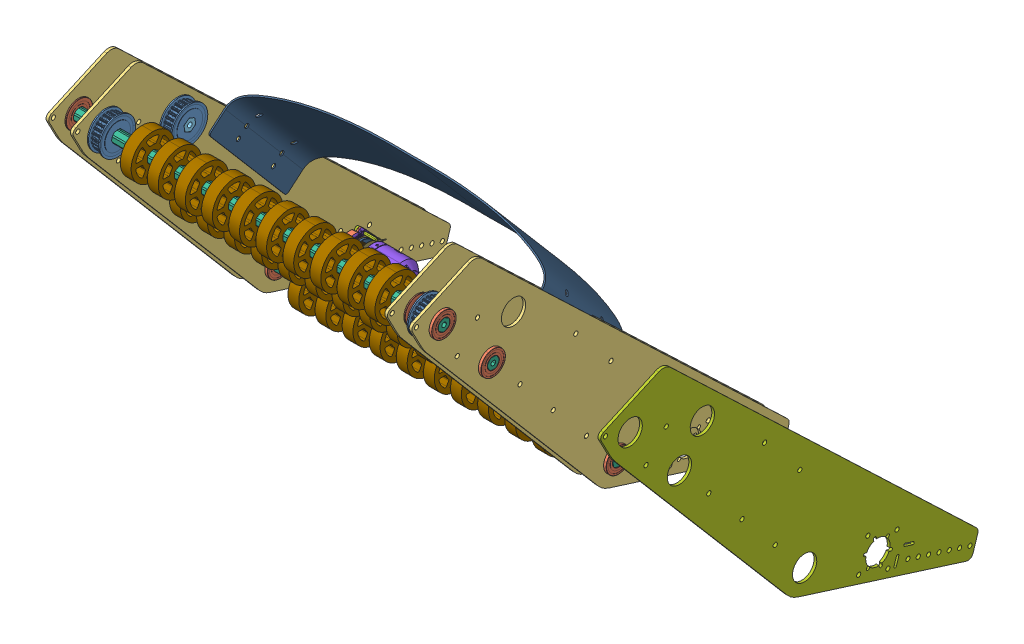
SolidWorks assembly noahbackupintake, configuration Default. Lengths in mm.
Overall size (656.48 502.65 458.04).
111 component instances, 28 part files, 0 mates.
Components (placement in the parent):
- EBUD-000_INTAKE_STEP_ASM^04_INTAKE_ASM_00_2023_everybot_asm_final_rev2(2)_00_2023_everybot_asm_final_rev2-1: EBUD-000_INTAKE_STEP_ASM^04_INTAKE_ASM_00_2023_everybot_asm_final_rev2(2)_00_2023_everybot_asm_final_rev2 [Default] at origin size (656.48 502.65 458.04) (virtual)
  - 24T_X_9MM_WIDE_DOUBLE_FLANGE_AL^EBUD-000_INTAKE_STEP_ASM_04_INTAKE_ASM_00_2023_everybot_asm_final_rev2(2)_00_2023_everybot_asm_final_rev2-1: 24T_X_9MM_WIDE_DOUBLE_FLANGE_AL^EBUD-000_INTAKE_STEP_ASM_04_INTAKE_ASM_00_2023_everybot_asm_final_rev2(2)_00_2023_everybot_asm_final_rev2 [Default] at (-209.55 741.6884 782.7658) x (0 0.711961 0.702219) z (1 0 0) size (42 42 14.5) (virtual)
  - 24T_X_9MM_WIDE_DOUBLE_FLANGE_AL^EBUD-000_INTAKE_STEP_ASM_04_INTAKE_ASM_00_2023_everybot_asm_final_rev2(2)_00_2023_everybot_asm_final_rev2-2: 24T_X_9MM_WIDE_DOUBLE_FLANGE_AL^EBUD-000_INTAKE_STEP_ASM_04_INTAKE_ASM_00_2023_everybot_asm_final_rev2(2)_00_2023_everybot_asm_final_rev2 [Default] at (-209.55 714.5782 696.9507) x (0 -0.172794 -0.984958) z (1 0 0) size (42 42 14.5) (virtual)
  - 13_75MM__1_2_THUNDERHEX_ID__X_1^EBUD-000_INTAKE_STEP_ASM_04_INTAKE_ASM_00_2023_everybot_asm_final_rev2(2)_00_2023_everybot_asm_final_rev2-1: 13_75MM__1_2_THUNDERHEX_ID__X_1^EBUD-000_INTAKE_STEP_ASM_04_INTAKE_ASM_00_2023_everybot_asm_final_rev2(2)_00_2023_everybot_asm_final_rev2 [Default] at (-224.6312 714.5782 696.9507) x (0 -0.939164 0.343468) z (1 0 0) size (31.12 31.12 7.94) (virtual)
  - 13_75MM__1_2_THUNDERHEX_ID__X_1^EBUD-000_INTAKE_STEP_ASM_04_INTAKE_ASM_00_2023_everybot_asm_final_rev2(2)_00_2023_everybot_asm_final_rev2-2: 13_75MM__1_2_THUNDERHEX_ID__X_1^EBUD-000_INTAKE_STEP_ASM_04_INTAKE_ASM_00_2023_everybot_asm_final_rev2(2)_00_2023_everybot_asm_final_rev2 [Default] at (-224.6312 741.6884 782.7658) x (0 -0.292473 -0.956274) z (1 0 0) size (31.12 31.12 7.94) (virtual)
  - 04_INTAKE_PLATE^EBUD-000_INTAKE_STEP_ASM_04_INTAKE_ASM_00_2023_everybot_asm_final_rev2(2)_00_2023_everybot_asm_final_rev2-1: 04_INTAKE_PLATE^EBUD-000_INTAKE_STEP_ASM_04_INTAKE_ASM_00_2023_everybot_asm_final_rev2(2)_00_2023_everybot_asm_final_rev2 [Default] at (-223.8375 981.3273 987.2051) x (1 0 0) z (0 -0.649023 0.760769) size (3.17 540.33 141.11) (virtual)
  - 04_INTAKE_PLATE^EBUD-000_INTAKE_STEP_ASM_04_INTAKE_ASM_00_2023_everybot_asm_final_rev2(2)_00_2023_everybot_asm_final_rev2-2: 04_INTAKE_PLATE^EBUD-000_INTAKE_STEP_ASM_04_INTAKE_ASM_00_2023_everybot_asm_final_rev2(2)_00_2023_everybot_asm_final_rev2 [Default] at (-195.2625 981.3273 987.2051) x (1 0 0) z (0 -0.649023 0.760769) size (3.17 540.33 141.11) (virtual)
  - 04_INTAKE_PLATE^EBUD-000_INTAKE_STEP_ASM_04_INTAKE_ASM_00_2023_everybot_asm_final_rev2(2)_00_2023_everybot_asm_final_rev2-3: 04_INTAKE_PLATE^EBUD-000_INTAKE_STEP_ASM_04_INTAKE_ASM_00_2023_everybot_asm_final_rev2(2)_00_2023_everybot_asm_final_rev2 [Default] at (173.1645 981.3273 987.2051) x (1 0 0) z (0 -0.649023 0.760769) size (3.17 540.33 141.11) (virtual)
  - 04_INTAKE_PLATE^EBUD-000_INTAKE_STEP_ASM_04_INTAKE_ASM_00_2023_everybot_asm_final_rev2(2)_00_2023_everybot_asm_final_rev2-4: 04_INTAKE_PLATE^EBUD-000_INTAKE_STEP_ASM_04_INTAKE_ASM_00_2023_everybot_asm_final_rev2(2)_00_2023_everybot_asm_final_rev2 [Default] at (201.7395 981.3273 987.2051) x (1 0 0) z (0 -0.649023 0.760769) size (3.17 540.33 141.11) (virtual)
  - 13_75MM__1_2_THUNDERHEX_ID__X_1^EBUD-000_INTAKE_STEP_ASM_04_INTAKE_ASM_00_2023_everybot_asm_final_rev2(2)_00_2023_everybot_asm_final_rev2-3: 13_75MM__1_2_THUNDERHEX_ID__X_1^EBUD-000_INTAKE_STEP_ASM_04_INTAKE_ASM_00_2023_everybot_asm_final_rev2(2)_00_2023_everybot_asm_final_rev2 [Default] at (-194.4688 981.3273 987.2051) x (0 0.254987 0.966944) z (-1 0 0) size (31.12 31.12 7.94) (virtual)
  - 13_75MM__1_2_THUNDERHEX_ID__X_1^EBUD-000_INTAKE_STEP_ASM_04_INTAKE_ASM_00_2023_everybot_asm_final_rev2(2)_00_2023_everybot_asm_final_rev2-4: 13_75MM__1_2_THUNDERHEX_ID__X_1^EBUD-000_INTAKE_STEP_ASM_04_INTAKE_ASM_00_2023_everybot_asm_final_rev2(2)_00_2023_everybot_asm_final_rev2 [Default] at (-224.6312 950.6568 902.5971) x (0 0.861369 0.50798) z (1 0 0) size (31.12 31.12 7.94) (virtual)
  - 13_75MM__1_2_THUNDERHEX_ID__X_1^EBUD-000_INTAKE_STEP_ASM_04_INTAKE_ASM_00_2023_everybot_asm_final_rev2(2)_00_2023_everybot_asm_final_rev2-5: 13_75MM__1_2_THUNDERHEX_ID__X_1^EBUD-000_INTAKE_STEP_ASM_04_INTAKE_ASM_00_2023_everybot_asm_final_rev2(2)_00_2023_everybot_asm_final_rev2 [Default] at (-224.6312 981.3273 987.2051) x (0 0.96991 0.243463) z (1 0 0) size (31.12 31.12 7.94) (virtual)
  - 24T_X_9MM_WIDE_DOUBLE_FLANGE_AL^EBUD-000_INTAKE_STEP_ASM_04_INTAKE_ASM_00_2023_everybot_asm_final_rev2(2)_00_2023_everybot_asm_final_rev2-3: 24T_X_9MM_WIDE_DOUBLE_FLANGE_AL^EBUD-000_INTAKE_STEP_ASM_04_INTAKE_ASM_00_2023_everybot_asm_final_rev2(2)_00_2023_everybot_asm_final_rev2 [Default] at (-183.25 981.3273 987.2051) x (0 -0.068988 0.997618) z (1 0 0) size (42 42 14.5) (virtual)
  - 13_75MM__1_2_THUNDERHEX_ID__X_1^EBUD-000_INTAKE_STEP_ASM_04_INTAKE_ASM_00_2023_everybot_asm_final_rev2(2)_00_2023_everybot_asm_final_rev2-6: 13_75MM__1_2_THUNDERHEX_ID__X_1^EBUD-000_INTAKE_STEP_ASM_04_INTAKE_ASM_00_2023_everybot_asm_final_rev2(2)_00_2023_everybot_asm_final_rev2 [Default] at (-194.4688 913.695 929.507) x (0 0.294166 0.955754) z (-1 0 0) size (31.12 31.12 7.94) (virtual)
  - 13_75MM__1_2_THUNDERHEX_ID__X_1^EBUD-000_INTAKE_STEP_ASM_04_INTAKE_ASM_00_2023_everybot_asm_final_rev2(2)_00_2023_everybot_asm_final_rev2-7: 13_75MM__1_2_THUNDERHEX_ID__X_1^EBUD-000_INTAKE_STEP_ASM_04_INTAKE_ASM_00_2023_everybot_asm_final_rev2(2)_00_2023_everybot_asm_final_rev2 [Default] at (-224.6312 913.695 929.507) x (0 0.91904 0.394165) z (1 0 0) size (31.12 31.12 7.94) (virtual)
  - REV-21-1929^EBUD-000_INTAKE_STEP_ASM_04_INTAKE_ASM_00_2023_everybot_asm_final_rev2(2)_00_2023_everybot_asm_final_rev2-1: REV-21-1929^EBUD-000_INTAKE_STEP_ASM_04_INTAKE_ASM_00_2023_everybot_asm_final_rev2(2)_00_2023_everybot_asm_final_rev2 [Default] at (-209.55 913.695 929.507) x (0 0 1) z (-1 0 0) size (48.2 48.2 12.7) (virtual)
  - 13_75MM__1_2_THUNDERHEX_ID__X_1^EBUD-000_INTAKE_STEP_ASM_04_INTAKE_ASM_00_2023_everybot_asm_final_rev2(2)_00_2023_everybot_asm_final_rev2-8: 13_75MM__1_2_THUNDERHEX_ID__X_1^EBUD-000_INTAKE_STEP_ASM_04_INTAKE_ASM_00_2023_everybot_asm_final_rev2(2)_00_2023_everybot_asm_final_rev2 [Default] at (-194.4688 741.6884 782.7658) x (0 -0.454664 -0.890663) z (-1 0 0) size (31.12 31.12 7.94) (virtual)
  - REV-21-1929^EBUD-000_INTAKE_STEP_ASM_04_INTAKE_ASM_00_2023_everybot_asm_final_rev2(2)_00_2023_everybot_asm_final_rev2-2: REV-21-1929^EBUD-000_INTAKE_STEP_ASM_04_INTAKE_ASM_00_2023_everybot_asm_final_rev2(2)_00_2023_everybot_asm_final_rev2 [Default] at (-209.55 950.6568 902.5971) x (0 0.397418 0.917638) z (-1 0 0) size (48.2 48.2 12.7) (virtual)
  - 13_75MM__1_2_THUNDERHEX_ID__X_1^EBUD-000_INTAKE_STEP_ASM_04_INTAKE_ASM_00_2023_everybot_asm_final_rev2(2)_00_2023_everybot_asm_final_rev2-9: 13_75MM__1_2_THUNDERHEX_ID__X_1^EBUD-000_INTAKE_STEP_ASM_04_INTAKE_ASM_00_2023_everybot_asm_final_rev2(2)_00_2023_everybot_asm_final_rev2 [Default] at (-194.4688 950.6568 902.5971) x (0 0.163432 0.986555) z (-1 0 0) size (31.12 31.12 7.94) (virtual)
  - 24T_X_9MM_WIDE_DOUBLE_FLANGE_AL^EBUD-000_INTAKE_STEP_ASM_04_INTAKE_ASM_00_2023_everybot_asm_final_rev2(2)_00_2023_everybot_asm_final_rev2-4: 24T_X_9MM_WIDE_DOUBLE_FLANGE_AL^EBUD-000_INTAKE_STEP_ASM_04_INTAKE_ASM_00_2023_everybot_asm_final_rev2(2)_00_2023_everybot_asm_final_rev2 [Default] at (-183.25 950.6568 902.5971) x (0 0.99517 0.098168) z (1 0 0) size (42 42 14.5) (virtual)
  - 13_75MM__1_2_THUNDERHEX_ID__X_1^EBUD-000_INTAKE_STEP_ASM_04_INTAKE_ASM_00_2023_everybot_asm_final_rev2(2)_00_2023_everybot_asm_final_rev2-10: 13_75MM__1_2_THUNDERHEX_ID__X_1^EBUD-000_INTAKE_STEP_ASM_04_INTAKE_ASM_00_2023_everybot_asm_final_rev2(2)_00_2023_everybot_asm_final_rev2 [Default] at (172.3707 913.695 929.507) x (0 -0.294166 -0.955754) z (1 0 0) size (31.12 31.12 7.94) (virtual)
  - 13_75MM__1_2_THUNDERHEX_ID__X_1^EBUD-000_INTAKE_STEP_ASM_04_INTAKE_ASM_00_2023_everybot_asm_final_rev2(2)_00_2023_everybot_asm_final_rev2-11: 13_75MM__1_2_THUNDERHEX_ID__X_1^EBUD-000_INTAKE_STEP_ASM_04_INTAKE_ASM_00_2023_everybot_asm_final_rev2(2)_00_2023_everybot_asm_final_rev2 [Default] at (172.3707 741.6884 782.7658) x (0 0.454664 0.890663) z (1 0 0) size (31.12 31.12 7.94) (virtual)
  - 13_75MM__1_2_THUNDERHEX_ID__X_1^EBUD-000_INTAKE_STEP_ASM_04_INTAKE_ASM_00_2023_everybot_asm_final_rev2(2)_00_2023_everybot_asm_final_rev2-12: 13_75MM__1_2_THUNDERHEX_ID__X_1^EBUD-000_INTAKE_STEP_ASM_04_INTAKE_ASM_00_2023_everybot_asm_final_rev2(2)_00_2023_everybot_asm_final_rev2 [Default] at (202.5333 981.3273 987.2051) x (0 -0.96991 -0.243463) z (-1 0 0) size (31.12 31.12 7.94) (virtual)
  - 13_75MM__1_2_THUNDERHEX_ID__X_1^EBUD-000_INTAKE_STEP_ASM_04_INTAKE_ASM_00_2023_everybot_asm_final_rev2(2)_00_2023_everybot_asm_final_rev2-13: 13_75MM__1_2_THUNDERHEX_ID__X_1^EBUD-000_INTAKE_STEP_ASM_04_INTAKE_ASM_00_2023_everybot_asm_final_rev2(2)_00_2023_everybot_asm_final_rev2 [Default] at (202.5333 913.695 929.507) x (0 -0.91904 -0.394165) z (-1 0 0) size (31.12 31.12 7.94) (virtual)
  - 13_75MM__1_2_THUNDERHEX_ID__X_1^EBUD-000_INTAKE_STEP_ASM_04_INTAKE_ASM_00_2023_everybot_asm_final_rev2(2)_00_2023_everybot_asm_final_rev2-14: 13_75MM__1_2_THUNDERHEX_ID__X_1^EBUD-000_INTAKE_STEP_ASM_04_INTAKE_ASM_00_2023_everybot_asm_final_rev2(2)_00_2023_everybot_asm_final_rev2 [Default] at (202.5333 741.6884 782.7658) x (0 0.292473 0.956274) z (-1 0 0) size (31.12 31.12 7.94) (virtual)
  - 13_75MM__1_2_THUNDERHEX_ID__X_1^EBUD-000_INTAKE_STEP_ASM_04_INTAKE_ASM_00_2023_everybot_asm_final_rev2(2)_00_2023_everybot_asm_final_rev2-15: 13_75MM__1_2_THUNDERHEX_ID__X_1^EBUD-000_INTAKE_STEP_ASM_04_INTAKE_ASM_00_2023_everybot_asm_final_rev2(2)_00_2023_everybot_asm_final_rev2 [Default] at (172.3707 981.3273 987.2051) x (0 -0.254987 -0.966944) z (1 0 0) size (31.12 31.12 7.94) (virtual)
  - 04_CLUSTER_SHAFT^EBUD-000_INTAKE_STEP_ASM_04_INTAKE_ASM_00_2023_everybot_asm_final_rev2(2)_00_2023_everybot_asm_final_rev2-1: 04_CLUSTER_SHAFT^EBUD-000_INTAKE_STEP_ASM_04_INTAKE_ASM_00_2023_everybot_asm_final_rev2(2)_00_2023_everybot_asm_final_rev2 [Default] at (-190.605 950.6568 902.5971) x (1 0 0) z (0 0.754856 0.65589) size (55.88 13.76 12.7) (virtual)
  - 24T_X_9MM_WIDE_DOUBLE_FLANGE_AL^EBUD-000_INTAKE_STEP_ASM_04_INTAKE_ASM_00_2023_everybot_asm_final_rev2(2)_00_2023_everybot_asm_final_rev2-5: 24T_X_9MM_WIDE_DOUBLE_FLANGE_AL^EBUD-000_INTAKE_STEP_ASM_04_INTAKE_ASM_00_2023_everybot_asm_final_rev2(2)_00_2023_everybot_asm_final_rev2 [Default] at (191.3145 741.6884 782.7658) x (0 -0.01901 0.999819) z (1 0 0) size (42 42 14.5) (virtual)
  - 24T_X_9MM_WIDE_DOUBLE_FLANGE_AL^EBUD-000_INTAKE_STEP_ASM_04_INTAKE_ASM_00_2023_everybot_asm_final_rev2(2)_00_2023_everybot_asm_final_rev2-6: 24T_X_9MM_WIDE_DOUBLE_FLANGE_AL^EBUD-000_INTAKE_STEP_ASM_04_INTAKE_ASM_00_2023_everybot_asm_final_rev2(2)_00_2023_everybot_asm_final_rev2 [Default] at (191.3145 981.3273 987.2051) x (0 -0.068988 0.997618) z (1 0 0) size (42 42 14.5) (virtual)
  - 04_INTAKE_ROLLER_SHAFT^EBUD-000_INTAKE_STEP_ASM_04_INTAKE_ASM_00_2023_everybot_asm_final_rev2(2)_00_2023_everybot_asm_final_rev2-1: 04_INTAKE_ROLLER_SHAFT^EBUD-000_INTAKE_STEP_ASM_04_INTAKE_ASM_00_2023_everybot_asm_final_rev2(2)_00_2023_everybot_asm_final_rev2 [Default] at (-37.973 741.6873 782.7662) x (1 0 0) z (0 -0.958269 0.285869) size (435.1 13.76 12.7) (virtual)
  - 04_INTAKE_ROLLER_SHAFT^EBUD-000_INTAKE_STEP_ASM_04_INTAKE_ASM_00_2023_everybot_asm_final_rev2(2)_00_2023_everybot_asm_final_rev2-2: 04_INTAKE_ROLLER_SHAFT^EBUD-000_INTAKE_STEP_ASM_04_INTAKE_ASM_00_2023_everybot_asm_final_rev2(2)_00_2023_everybot_asm_final_rev2 [Default] at (-37.973 913.695 929.507) x (1 0 0) z (0 -0.53426 -0.84532) size (435.1 13.76 12.7) (virtual)
  - 04_INTAKE_ROLLER_SHAFT^EBUD-000_INTAKE_STEP_ASM_04_INTAKE_ASM_00_2023_everybot_asm_final_rev2(2)_00_2023_everybot_asm_final_rev2-3: 04_INTAKE_ROLLER_SHAFT^EBUD-000_INTAKE_STEP_ASM_04_INTAKE_ASM_00_2023_everybot_asm_final_rev2(2)_00_2023_everybot_asm_final_rev2 [Default] at (-37.973 981.3273 987.2051) size (435.1 13.76 12.7) (virtual)
  - 04_INTAKE_PLATE_REV2_REF_ONLY^EBUD-000_INTAKE_STEP_ASM_04_INTAKE_ASM_00_2023_everybot_asm_final_rev2(2)_00_2023_everybot_asm_final_rev2-1: 04_INTAKE_PLATE_REV2_REF_ONLY^EBUD-000_INTAKE_STEP_ASM_04_INTAKE_ASM_00_2023_everybot_asm_final_rev2(2)_00_2023_everybot_asm_final_rev2 [Default] at (423.0079 981.3273 987.2051) x (1 0 0) z (0 -0.649023 0.760769) size (3.17 540.33 141.11) (virtual)
- REV_ULTRAPLANETARY_1-STAGE_ASM^04_INTAKE_ASM_00_2023_everybot_asm_final_rev2(2)_00_2023_everybot_asm_final_rev2-1: REV_ULTRAPLANETARY_1-STAGE_ASM^04_INTAKE_ASM_00_2023_everybot_asm_final_rev2(2)_00_2023_everybot_asm_final_rev2 [Default] at (-167.425 714.5782 696.9507) x (0 -0.976417 -0.215894) z (1 0 0) size (56.74 54.7 105.61) (virtual)
  - REV_ULTRAPLANETARY__CONFIGURABL_ASM^REV_ULTRAPLANETARY_1-STAGE_ASM_04_INTAKE_ASM_00_2023_everybot_asm_final_rev2(2)_00_2023_everybot_asm_final_rev2-1: REV_ULTRAPLANETARY__CONFIGURABL_ASM^REV_ULTRAPLANETARY_1-STAGE_ASM_04_INTAKE_ASM_00_2023_everybot_asm_final_rev2(2)_00_2023_everybot_asm_final_rev2 [Default] at origin size (56.74 54.7 105.61) (virtual)
    - REV_PLANETARY_STAGE__1__ASM^REV_ULTRAPLANETARY__CONFIGURABL_ASM_REV_ULTRAPLANETARY_1-STAGE_ASM_04_INTAKE_ASM_00_2023_everybot_asm_final_rev2(2)_00_2023_everybot_asm_final_rev2-1: REV_PLANETARY_STAGE__1__ASM^REV_ULTRAPLANETARY__CONFIGURABL_ASM_REV_ULTRAPLANETARY_1-STAGE_ASM_04_INTAKE_ASM_00_2023_everybot_asm_final_rev2(2)_00_2023_everybot_asm_final_rev2 [Default] at origin size (47.64 47.49 16.75) (virtual)
      - REV_ULTRAPLANETARY_3_1_CARTRIDG_ASM^REV_PLANETARY_STAGE__1__ASM_REV_ULTRAPLANETARY__CONFIGURABL_ASM_REV_ULTRAPLANETARY_1-STAGE_ASM_04_INTAKE_ASM_00_2023_everybot_asm_final_rev2(2)_00_2023~-1: REV_ULTRAPLANETARY_3_1_CARTRIDG_ASM^REV_PLANETARY_STAGE__1__ASM_REV_ULTRAPLANETARY__CONFIGURABL_ASM_REV_ULTRAPLANETARY_1-STAGE_ASM_04_INTAKE_ASM_00_2023_everybot_asm_final_rev2(2)_00_2023_~ [Default] at origin size (47.64 47.49 16.75) (virtual)
        - REV-40-1613^REV_ULTRAPLANETARY_3_1_CARTRIDG_ASM_REV_PLANETARY_STAGE__1__ASM_REV_ULTRAPLANETARY__CONFIGURABL_ASM_REV_ULTRAPLANETARY_1-STAGE_ASM_04_INTAKE_ASM_00_2023_everybot_asm_final_rev2~-1: REV-40-1613^REV_ULTRAPLANETARY_3_1_CARTRIDG_ASM_REV_PLANETARY_STAGE__1__ASM_REV_ULTRAPLANETARY__CONFIGURABL_ASM_REV_ULTRAPLANETARY_1-STAGE_ASM_04_INTAKE_ASM_00_2023_everybot_asm_final_rev2~ [Default] at (-0.89 11.5157 -14.625) x (0 0 1) z (-0.923728 -0.383049 0) size (9 3 3) (virtual)
        - REV-41-1601-2^REV_ULTRAPLANETARY_3_1_CARTRIDG_ASM_REV_PLANETARY_STAGE__1__ASM_REV_ULTRAPLANETARY__CONFIGURABL_ASM_REV_ULTRAPLANETARY_1-STAGE_ASM_04_INTAKE_ASM_00_2023_everybot_asm_final_re~-1: REV-41-1601-2^REV_ULTRAPLANETARY_3_1_CARTRIDG_ASM_REV_PLANETARY_STAGE__1__ASM_REV_ULTRAPLANETARY__CONFIGURABL_ASM_REV_ULTRAPLANETARY_1-STAGE_ASM_04_INTAKE_ASM_00_2023_everybot_asm_final_re~ [Default] at (-0.89 11.5157 -8.625) x (0.281273 0.959628 0) z (0.959628 -0.281273 0) size (8.22 6.01 8.17) (virtual)
        - REV-41-1601-2^REV_ULTRAPLANETARY_3_1_CARTRIDG_ASM_REV_PLANETARY_STAGE__1__ASM_REV_ULTRAPLANETARY__CONFIGURABL_ASM_REV_ULTRAPLANETARY_1-STAGE_ASM_04_INTAKE_ASM_00_2023_everybot_asm_final_re~-2: REV-41-1601-2^REV_ULTRAPLANETARY_3_1_CARTRIDG_ASM_REV_PLANETARY_STAGE__1__ASM_REV_ULTRAPLANETARY__CONFIGURABL_ASM_REV_ULTRAPLANETARY_1-STAGE_ASM_04_INTAKE_ASM_00_2023_everybot_asm_final_re~ [Default] at (-11.5157 -0.89 -8.625) x (0.938661 0.34484 0) z (0.34484 -0.938661 0) size (8.22 6.01 8.17) (virtual)
        - REV-40-1613^REV_ULTRAPLANETARY_3_1_CARTRIDG_ASM_REV_PLANETARY_STAGE__1__ASM_REV_ULTRAPLANETARY__CONFIGURABL_ASM_REV_ULTRAPLANETARY_1-STAGE_ASM_04_INTAKE_ASM_00_2023_everybot_asm_final_rev2~-2: REV-40-1613^REV_ULTRAPLANETARY_3_1_CARTRIDG_ASM_REV_PLANETARY_STAGE__1__ASM_REV_ULTRAPLANETARY__CONFIGURABL_ASM_REV_ULTRAPLANETARY_1-STAGE_ASM_04_INTAKE_ASM_00_2023_everybot_asm_final_rev2~ [Default] at (0.89 -11.5157 -14.625) x (0 0 1) z (-0.923728 -0.383049 0) size (9 3 3) (virtual)
        - REV-40-1613^REV_ULTRAPLANETARY_3_1_CARTRIDG_ASM_REV_PLANETARY_STAGE__1__ASM_REV_ULTRAPLANETARY__CONFIGURABL_ASM_REV_ULTRAPLANETARY_1-STAGE_ASM_04_INTAKE_ASM_00_2023_everybot_asm_final_rev2~-3: REV-40-1613^REV_ULTRAPLANETARY_3_1_CARTRIDG_ASM_REV_PLANETARY_STAGE__1__ASM_REV_ULTRAPLANETARY__CONFIGURABL_ASM_REV_ULTRAPLANETARY_1-STAGE_ASM_04_INTAKE_ASM_00_2023_everybot_asm_final_rev2~ [Default] at (11.5157 0.89 -14.625) x (0 0 1) z (-0.923728 -0.383049 0) size (9 3 3) (virtual)
        - REV-41-1601-1^REV_ULTRAPLANETARY_3_1_CARTRIDG_ASM_REV_PLANETARY_STAGE__1__ASM_REV_ULTRAPLANETARY__CONFIGURABL_ASM_REV_ULTRAPLANETARY_1-STAGE_ASM_04_INTAKE_ASM_00_2023_everybot_asm_final_re~-1: REV-41-1601-1^REV_ULTRAPLANETARY_3_1_CARTRIDG_ASM_REV_PLANETARY_STAGE__1__ASM_REV_ULTRAPLANETARY__CONFIGURABL_ASM_REV_ULTRAPLANETARY_1-STAGE_ASM_04_INTAKE_ASM_00_2023_everybot_asm_final_re~ [Default] at (0 0 -11.875) x (0.997027 0.077058 0) z (0 0 -1) size (29.1 29.1 10.25) (virtual)
        - REV-41-1601-2^REV_ULTRAPLANETARY_3_1_CARTRIDG_ASM_REV_PLANETARY_STAGE__1__ASM_REV_ULTRAPLANETARY__CONFIGURABL_ASM_REV_ULTRAPLANETARY_1-STAGE_ASM_04_INTAKE_ASM_00_2023_everybot_asm_final_re~-3: REV-41-1601-2^REV_ULTRAPLANETARY_3_1_CARTRIDG_ASM_REV_PLANETARY_STAGE__1__ASM_REV_ULTRAPLANETARY__CONFIGURABL_ASM_REV_ULTRAPLANETARY_1-STAGE_ASM_04_INTAKE_ASM_00_2023_everybot_asm_final_re~ [Default] at (0.89 -11.5157 -8.625) x (0.79716 -0.603767 0) z (-0.603767 -0.79716 0) size (8.22 6.01 8.17) (virtual)
        - REV-41-1601-3^REV_ULTRAPLANETARY_3_1_CARTRIDG_ASM_REV_PLANETARY_STAGE__1__ASM_REV_ULTRAPLANETARY__CONFIGURABL_ASM_REV_ULTRAPLANETARY_1-STAGE_ASM_04_INTAKE_ASM_00_2023_everybot_asm_final_re~-1: REV-41-1601-3^REV_ULTRAPLANETARY_3_1_CARTRIDG_ASM_REV_PLANETARY_STAGE__1__ASM_REV_ULTRAPLANETARY__CONFIGURABL_ASM_REV_ULTRAPLANETARY_1-STAGE_ASM_04_INTAKE_ASM_00_2023_everybot_asm_final_re~ [Default] at (0 0 -8.75) x (-0.670912 -0.741537 0) z (-0.741537 0.670912 0) size (17.04 6.01 17.02) (virtual)
        - REV-40-1619^REV_ULTRAPLANETARY_3_1_CARTRIDG_ASM_REV_PLANETARY_STAGE__1__ASM_REV_ULTRAPLANETARY__CONFIGURABL_ASM_REV_ULTRAPLANETARY_1-STAGE_ASM_04_INTAKE_ASM_00_2023_everybot_asm_final_rev2~-1: REV-40-1619^REV_ULTRAPLANETARY_3_1_CARTRIDG_ASM_REV_PLANETARY_STAGE__1__ASM_REV_ULTRAPLANETARY__CONFIGURABL_ASM_REV_ULTRAPLANETARY_1-STAGE_ASM_04_INTAKE_ASM_00_2023_everybot_asm_final_rev2~ [Default] at (0 0 -14.875) x (-0.866025 -0.5 0) z (0 0 -1) size (35.02 34.62 3.62) (virtual)
        - REV-40-1619^REV_ULTRAPLANETARY_3_1_CARTRIDG_ASM_REV_PLANETARY_STAGE__1__ASM_REV_ULTRAPLANETARY__CONFIGURABL_ASM_REV_ULTRAPLANETARY_1-STAGE_ASM_04_INTAKE_ASM_00_2023_everybot_asm_final_rev2~-2: REV-40-1619^REV_ULTRAPLANETARY_3_1_CARTRIDG_ASM_REV_PLANETARY_STAGE__1__ASM_REV_ULTRAPLANETARY__CONFIGURABL_ASM_REV_ULTRAPLANETARY_1-STAGE_ASM_04_INTAKE_ASM_00_2023_everybot_asm_final_rev2~ [Default] at (0 0 -5.125) x (0 -1 0) z (0 0 1) size (35.02 34.62 3.62) (virtual)
        - REV-40-1613^REV_ULTRAPLANETARY_3_1_CARTRIDG_ASM_REV_PLANETARY_STAGE__1__ASM_REV_ULTRAPLANETARY__CONFIGURABL_ASM_REV_ULTRAPLANETARY_1-STAGE_ASM_04_INTAKE_ASM_00_2023_everybot_asm_final_rev2~-4: REV-40-1613^REV_ULTRAPLANETARY_3_1_CARTRIDG_ASM_REV_PLANETARY_STAGE__1__ASM_REV_ULTRAPLANETARY__CONFIGURABL_ASM_REV_ULTRAPLANETARY_1-STAGE_ASM_04_INTAKE_ASM_00_2023_everybot_asm_final_rev2~ [Default] at (-11.5157 -0.89 -14.625) x (0 0 1) z (-0.923728 -0.383049 0) size (9 3 3) (virtual)
        - REV-41-1601-2^REV_ULTRAPLANETARY_3_1_CARTRIDG_ASM_REV_PLANETARY_STAGE__1__ASM_REV_ULTRAPLANETARY__CONFIGURABL_ASM_REV_ULTRAPLANETARY_1-STAGE_ASM_04_INTAKE_ASM_00_2023_everybot_asm_final_re~-4: REV-41-1601-2^REV_ULTRAPLANETARY_3_1_CARTRIDG_ASM_REV_PLANETARY_STAGE__1__ASM_REV_ULTRAPLANETARY__CONFIGURABL_ASM_REV_ULTRAPLANETARY_1-STAGE_ASM_04_INTAKE_ASM_00_2023_everybot_asm_final_re~ [Default] at (11.5157 0.89 -8.625) x (0.79726 -0.603636 0) z (-0.603636 -0.79726 0) size (8.22 6.01 8.17) (virtual)
    - REV_ULTRAPLANETARY_OUTPUT_STAGE_ASM^REV_ULTRAPLANETARY__CONFIGURABL_ASM_REV_ULTRAPLANETARY_1-STAGE_ASM_04_INTAKE_ASM_00_2023_everybot_asm_final_rev2(2)_00_2023_everybot_asm_final_rev2-1: REV_ULTRAPLANETARY_OUTPUT_STAGE_ASM^REV_ULTRAPLANETARY__CONFIGURABL_ASM_REV_ULTRAPLANETARY_1-STAGE_ASM_04_INTAKE_ASM_00_2023_everybot_asm_final_rev2(2)_00_2023_everybot_asm_final_rev2 [Default] at origin size (56.74 54.7 18.3) (virtual)
      - REV-41-1604-5^REV_ULTRAPLANETARY_OUTPUT_STAGE_ASM_REV_ULTRAPLANETARY__CONFIGURABL_ASM_REV_ULTRAPLANETARY_1-STAGE_ASM_04_INTAKE_ASM_00_2023_everybot_asm_final_rev2(2)_00_2023_everybot_asm_~-1: REV-41-1604-5^REV_ULTRAPLANETARY_OUTPUT_STAGE_ASM_REV_ULTRAPLANETARY__CONFIGURABL_ASM_REV_ULTRAPLANETARY_1-STAGE_ASM_04_INTAKE_ASM_00_2023_everybot_asm_final_rev2(2)_00_2023_everybot_asm_f~ [Default] at (0 0 -21.25) x (0.103978 -0.99458 0) z (0.99458 0.103978 0) size (23.5 0.75 23.5) (virtual)
      - SOCKET_HEAD_CAP_SCREW_AM_B18_3_^REV_ULTRAPLANETARY_OUTPUT_STAGE_ASM_REV_ULTRAPLANETARY__CONFIGURABL_ASM_REV_ULTRAPLANETARY_1-STAGE_ASM_04_INTAKE_ASM_00_2023_everybot_asm_final_rev2(2)_00_~-1: SOCKET_HEAD_CAP_SCREW_AM_B18_3_^REV_ULTRAPLANETARY_OUTPUT_STAGE_ASM_REV_ULTRAPLANETARY__CONFIGURABL_ASM_REV_ULTRAPLANETARY_1-STAGE_ASM_04_INTAKE_ASM_00_2023_everybot_asm_final_rev2(2)_00_2~ [Default] at (15.6357 3.3948 -15.05) x (0 0 -1) z (-0.934724 -0.355374 0) size (6 3.8 3.8) (virtual)
      - MCMASTER-CARR_91292A004_91292A0^REV_ULTRAPLANETARY_OUTPUT_STAGE_ASM_REV_ULTRAPLANETARY__CONFIGURABL_ASM_REV_ULTRAPLANETARY_1-STAGE_ASM_04_INTAKE_ASM_00_2023_everybot_asm_final_rev2(2)_00_~-1: MCMASTER-CARR_91292A004_91292A0^REV_ULTRAPLANETARY_OUTPUT_STAGE_ASM_REV_ULTRAPLANETARY__CONFIGURABL_ASM_REV_ULTRAPLANETARY_1-STAGE_ASM_04_INTAKE_ASM_00_2023_everybot_asm_final_rev2(2)_00_2~ [Default] at (-3.715 6.4346 -21.5) x (-0.608447 -0.793594 0) z (-0.793594 0.608447 0) size (3.8 6 3.8) (virtual)
      - 6704ZZ^REV_ULTRAPLANETARY_OUTPUT_STAGE_ASM_REV_ULTRAPLANETARY__CONFIGURABL_ASM_REV_ULTRAPLANETARY_1-STAGE_ASM_04_INTAKE_ASM_00_2023_everybot_asm_final_rev2(2)_00_2023_everybot_asm_final_r~-1: 6704ZZ^REV_ULTRAPLANETARY_OUTPUT_STAGE_ASM_REV_ULTRAPLANETARY__CONFIGURABL_ASM_REV_ULTRAPLANETARY_1-STAGE_ASM_04_INTAKE_ASM_00_2023_everybot_asm_final_rev2(2)_00_2023_everybot_asm_final_re~ [Default] at (0 0 -23.25) x (0.117109 -0.993119 0) z (0.993119 0.117109 0) size (27 4 27) (virtual)
      - 6704ZZ^REV_ULTRAPLANETARY_OUTPUT_STAGE_ASM_REV_ULTRAPLANETARY__CONFIGURABL_ASM_REV_ULTRAPLANETARY_1-STAGE_ASM_04_INTAKE_ASM_00_2023_everybot_asm_final_rev2(2)_00_2023_everybot_asm_final_r~-2: 6704ZZ^REV_ULTRAPLANETARY_OUTPUT_STAGE_ASM_REV_ULTRAPLANETARY__CONFIGURABL_ASM_REV_ULTRAPLANETARY_1-STAGE_ASM_04_INTAKE_ASM_00_2023_everybot_asm_final_rev2(2)_00_2023_everybot_asm_final_re~ [Default] at (0 0 -18.5) x (-0.099871 -0.995 0) z (0.995 -0.099871 0) size (27 4 27) (virtual)
      - MCMASTER-CARR_91292A004_91292A0^REV_ULTRAPLANETARY_OUTPUT_STAGE_ASM_REV_ULTRAPLANETARY__CONFIGURABL_ASM_REV_ULTRAPLANETARY_1-STAGE_ASM_04_INTAKE_ASM_00_2023_everybot_asm_final_rev2(2)_00_~-2: MCMASTER-CARR_91292A004_91292A0^REV_ULTRAPLANETARY_OUTPUT_STAGE_ASM_REV_ULTRAPLANETARY__CONFIGURABL_ASM_REV_ULTRAPLANETARY_1-STAGE_ASM_04_INTAKE_ASM_00_2023_everybot_asm_final_rev2(2)_00_2~ [Default] at (-3.715 -6.4346 -21.5) x (0.991496 -0.130134 0) z (-0.130134 -0.991496 0) size (3.8 6 3.8) (virtual)
      - MCMASTER-CARR_91292A004_91292A0^REV_ULTRAPLANETARY_OUTPUT_STAGE_ASM_REV_ULTRAPLANETARY__CONFIGURABL_ASM_REV_ULTRAPLANETARY_1-STAGE_ASM_04_INTAKE_ASM_00_2023_everybot_asm_final_rev2(2)_00_~-3: MCMASTER-CARR_91292A004_91292A0^REV_ULTRAPLANETARY_OUTPUT_STAGE_ASM_REV_ULTRAPLANETARY__CONFIGURABL_ASM_REV_ULTRAPLANETARY_1-STAGE_ASM_04_INTAKE_ASM_00_2023_everybot_asm_final_rev2(2)_00_2~ [Default] at (7.43 0 -21.5) x (-0.383049 0.923728 0) z (0.923728 0.383049 0) size (3.8 6 3.8) (virtual)
      - SOCKET_HEAD_CAP_SCREW_AM_B18_3_^REV_ULTRAPLANETARY_OUTPUT_STAGE_ASM_REV_ULTRAPLANETARY__CONFIGURABL_ASM_REV_ULTRAPLANETARY_1-STAGE_ASM_04_INTAKE_ASM_00_2023_everybot_asm_final_rev2(2)_00_~-2: SOCKET_HEAD_CAP_SCREW_AM_B18_3_^REV_ULTRAPLANETARY_OUTPUT_STAGE_ASM_REV_ULTRAPLANETARY__CONFIGURABL_ASM_REV_ULTRAPLANETARY_1-STAGE_ASM_04_INTAKE_ASM_00_2023_everybot_asm_final_rev2(2)_00_2~ [Default] at (-10.7579 11.8435 -15.05) x (0 0 -1) z (-0.492915 -0.870077 0) size (6 3.8 3.8) (virtual)
      - REV-41-1604-2^REV_ULTRAPLANETARY_OUTPUT_STAGE_ASM_REV_ULTRAPLANETARY__CONFIGURABL_ASM_REV_ULTRAPLANETARY_1-STAGE_ASM_04_INTAKE_ASM_00_2023_everybot_asm_final_rev2(2)_00_2023_everybot_asm_~-1: REV-41-1604-2^REV_ULTRAPLANETARY_OUTPUT_STAGE_ASM_REV_ULTRAPLANETARY__CONFIGURABL_ASM_REV_ULTRAPLANETARY_1-STAGE_ASM_04_INTAKE_ASM_00_2023_everybot_asm_final_rev2(2)_00_2023_everybot_asm_f~ [Default] at (0 0 -26.25) x (0 -1 0) z (1 0 0) size (43.57 6.3 38.01) (virtual)
      - REV-41-1611_THROUGH_HOLE^REV_ULTRAPLANETARY_OUTPUT_STAGE_ASM_REV_ULTRAPLANETARY__CONFIGURABL_ASM_REV_ULTRAPLANETARY_1-STAGE_ASM_04_INTAKE_ASM_00_2023_everybot_asm_final_rev2(2)_00_2023_ev~-1: REV-41-1611_THROUGH_HOLE^REV_ULTRAPLANETARY_OUTPUT_STAGE_ASM_REV_ULTRAPLANETARY__CONFIGURABL_ASM_REV_ULTRAPLANETARY_1-STAGE_ASM_04_INTAKE_ASM_00_2023_everybot_asm_final_rev2(2)_00_2023_eve~ [Default] at (0 0 -15.25) x (0 1 0) z (1 0 0) size (22 6.76 22) (virtual)
      - REV-41-1612^REV_ULTRAPLANETARY_OUTPUT_STAGE_ASM_REV_ULTRAPLANETARY__CONFIGURABL_ASM_REV_ULTRAPLANETARY_1-STAGE_ASM_04_INTAKE_ASM_00_2023_everybot_asm_final_rev2(2)_00_2023_everybot_asm_fi~-1: REV-41-1612^REV_ULTRAPLANETARY_OUTPUT_STAGE_ASM_REV_ULTRAPLANETARY__CONFIGURABL_ASM_REV_ULTRAPLANETARY_1-STAGE_ASM_04_INTAKE_ASM_00_2023_everybot_asm_final_rev2(2)_00_2023_everybot_asm_fin~ [Default] at (0 0 -19) x (-0.5 -0.866025 0) z (0 0 -1) size (22 21.65 13.25) (virtual)
      - REV-41-1604-1^REV_ULTRAPLANETARY_OUTPUT_STAGE_ASM_REV_ULTRAPLANETARY__CONFIGURABL_ASM_REV_ULTRAPLANETARY_1-STAGE_ASM_04_INTAKE_ASM_00_2023_everybot_asm_final_rev2(2)_00_2023_everybot_asm_~-1: REV-41-1604-1^REV_ULTRAPLANETARY_OUTPUT_STAGE_ASM_REV_ULTRAPLANETARY__CONFIGURABL_ASM_REV_ULTRAPLANETARY_1-STAGE_ASM_04_INTAKE_ASM_00_2023_everybot_asm_final_rev2(2)_00_2023_everybot_asm_f~ [Default] at (0 0 -19.25) x (0.866025 -0.5 0) z (-0.5 -0.866025 0) size (43.57 7.04 38.01) (virtual)
      - SOCKET_HEAD_CAP_SCREW_AM_B18_3_^REV_ULTRAPLANETARY_OUTPUT_STAGE_ASM_REV_ULTRAPLANETARY__CONFIGURABL_ASM_REV_ULTRAPLANETARY_1-STAGE_ASM_04_INTAKE_ASM_00_2023_everybot_asm_final_rev2(2)_00_~-3: SOCKET_HEAD_CAP_SCREW_AM_B18_3_^REV_ULTRAPLANETARY_OUTPUT_STAGE_ASM_REV_ULTRAPLANETARY__CONFIGURABL_ASM_REV_ULTRAPLANETARY_1-STAGE_ASM_04_INTAKE_ASM_00_2023_everybot_asm_final_rev2(2)_00_2~ [Default] at (-4.8778 -15.2383 -15.05) x (0 0 -1) z (0.970727 -0.240185 0) size (6 3.8 3.8) (virtual)
    - REV_ULTRAPLANETARY_550_MOTOR_PL_ASM^REV_ULTRAPLANETARY__CONFIGURABL_ASM_REV_ULTRAPLANETARY_1-STAGE_ASM_04_INTAKE_ASM_00_2023_everybot_asm_final_rev2(2)_00_2023_everybot_asm_final_rev2-1: REV_ULTRAPLANETARY_550_MOTOR_PL_ASM^REV_ULTRAPLANETARY__CONFIGURABL_ASM_REV_ULTRAPLANETARY_1-STAGE_ASM_04_INTAKE_ASM_00_2023_everybot_asm_final_rev2(2)_00_2023_everybot_asm_final_rev2 [Default] at origin size (9.12 31.6 16.65) (virtual)
      - REV-41-1608^REV_ULTRAPLANETARY_550_MOTOR_PL_ASM_REV_ULTRAPLANETARY__CONFIGURABL_ASM_REV_ULTRAPLANETARY_1-STAGE_ASM_04_INTAKE_ASM_00_2023_everybot_asm_final_rev2(2)_00_2023_everybot_asm_fi~-1: REV-41-1608^REV_ULTRAPLANETARY_550_MOTOR_PL_ASM_REV_ULTRAPLANETARY__CONFIGURABL_ASM_REV_ULTRAPLANETARY_1-STAGE_ASM_04_INTAKE_ASM_00_2023_everybot_asm_final_rev2(2)_00_2023_everybot_asm_fin~ [Default] at (0 0 -8) x (-0.123066 0.992399 0) z (0.992399 0.123066 0) size (8.22 7 8.17) (virtual)
      - M3X8_BUTTON_HEAD_91239A113^REV_ULTRAPLANETARY_550_MOTOR_PL_ASM_REV_ULTRAPLANETARY__CONFIGURABL_ASM_REV_ULTRAPLANETARY_1-STAGE_ASM_04_INTAKE_ASM_00_2023_everybot_asm_final_rev2(2)_00_2023_~-1: M3X8_BUTTON_HEAD_91239A113^REV_ULTRAPLANETARY_550_MOTOR_PL_ASM_REV_ULTRAPLANETARY__CONFIGURABL_ASM_REV_ULTRAPLANETARY_1-STAGE_ASM_04_INTAKE_ASM_00_2023_everybot_asm_final_rev2(2)_00_2023_e~ [Default] at (0.5 -12.49 -4.5) x (-0.04 0.9992 0) z (0.9992 0.04 0) size (5.7 9.66 5.7) (virtual)
      - M3X8_BUTTON_HEAD_91239A113^REV_ULTRAPLANETARY_550_MOTOR_PL_ASM_REV_ULTRAPLANETARY__CONFIGURABL_ASM_REV_ULTRAPLANETARY_1-STAGE_ASM_04_INTAKE_ASM_00_2023_everybot_asm_final_rev2(2)_00_2023_~-2: M3X8_BUTTON_HEAD_91239A113^REV_ULTRAPLANETARY_550_MOTOR_PL_ASM_REV_ULTRAPLANETARY__CONFIGURABL_ASM_REV_ULTRAPLANETARY_1-STAGE_ASM_04_INTAKE_ASM_00_2023_everybot_asm_final_rev2(2)_00_2023_e~ [Default] at (-0.5 12.49 -4.5) x (-0.938759 0.344575 0) z (0.344575 0.938759 0) size (5.7 9.66 5.7) (virtual)
    - HEX_SOCKET_HEAD_CAP_SCREW_M3X0_^REV_ULTRAPLANETARY__CONFIGURABL_ASM_REV_ULTRAPLANETARY_1-STAGE_ASM_04_INTAKE_ASM_00_2023_everybot_asm_final_rev2(2)_00_2023_everybot_asm_final_rev2-1: HEX_SOCKET_HEAD_CAP_SCREW_M3X0_^REV_ULTRAPLANETARY__CONFIGURABL_ASM_REV_ULTRAPLANETARY_1-STAGE_ASM_04_INTAKE_ASM_00_2023_everybot_asm_final_rev2(2)_00_2023_everybot_asm_final_rev2 [Default] at (6.9282 4 -38.25) x (-0.866025 0.5 0) z (0 0 -1) size (5.5 5.5 11) (virtual)
    - HEX_SOCKET_HEAD_CAP_SCREW_M3X0_^REV_ULTRAPLANETARY__CONFIGURABL_ASM_REV_ULTRAPLANETARY_1-STAGE_ASM_04_INTAKE_ASM_00_2023_everybot_asm_final_rev2(2)_00_2023_everybot_asm_final_rev2-2: HEX_SOCKET_HEAD_CAP_SCREW_M3X0_^REV_ULTRAPLANETARY__CONFIGURABL_ASM_REV_ULTRAPLANETARY_1-STAGE_ASM_04_INTAKE_ASM_00_2023_everybot_asm_final_rev2(2)_00_2023_everybot_asm_final_rev2 [Default] at (0 8 -38.25) x (-0.866025 -0.5 0) z (0 0 -1) size (5.5 5.5 11) (virtual)
    - UP_1_2__HEX_ADAPTER__REV-41-162^REV_ULTRAPLANETARY__CONFIGURABL_ASM_REV_ULTRAPLANETARY_1-STAGE_ASM_04_INTAKE_ASM_00_2023_everybot_asm_final_rev2(2)_00_2023_everybot_asm_final_rev2-1: UP_1_2__HEX_ADAPTER__REV-41-162^REV_ULTRAPLANETARY__CONFIGURABL_ASM_REV_ULTRAPLANETARY_1-STAGE_ASM_04_INTAKE_ASM_00_2023_everybot_asm_final_rev2(2)_00_2023_everybot_asm_final_rev2 [Default] at (0 0 -32.25) x (-0.5 -0.866025 0) z (0 0 1) size (22 22 30.59) (virtual)
    - HEX_SOCKET_HEAD_CAP_SCREW_M3X0_^REV_ULTRAPLANETARY__CONFIGURABL_ASM_REV_ULTRAPLANETARY_1-STAGE_ASM_04_INTAKE_ASM_00_2023_everybot_asm_final_rev2(2)_00_2023_everybot_asm_final_rev2-3: HEX_SOCKET_HEAD_CAP_SCREW_M3X0_^REV_ULTRAPLANETARY__CONFIGURABL_ASM_REV_ULTRAPLANETARY_1-STAGE_ASM_04_INTAKE_ASM_00_2023_everybot_asm_final_rev2(2)_00_2023_everybot_asm_final_rev2 [Default] at (0 -8 -38.25) x (0.866025 0.5 0) z (0 0 -1) size (5.5 5.5 11) (virtual)
    - HEX_SOCKET_HEAD_CAP_SCREW_M3X0_^REV_ULTRAPLANETARY__CONFIGURABL_ASM_REV_ULTRAPLANETARY_1-STAGE_ASM_04_INTAKE_ASM_00_2023_everybot_asm_final_rev2(2)_00_2023_everybot_asm_final_rev2-4: HEX_SOCKET_HEAD_CAP_SCREW_M3X0_^REV_ULTRAPLANETARY__CONFIGURABL_ASM_REV_ULTRAPLANETARY_1-STAGE_ASM_04_INTAKE_ASM_00_2023_everybot_asm_final_rev2(2)_00_2023_everybot_asm_final_rev2 [Default] at (-6.9282 -4 -38.25) x (0.866025 -0.5 0) z (0 0 -1) size (5.5 5.5 11) (virtual)
    - M3X40_91290A136^REV_ULTRAPLANETARY__CONFIGURABL_ASM_REV_ULTRAPLANETARY_1-STAGE_ASM_04_INTAKE_ASM_00_2023_everybot_asm_final_rev2(2)_00_2023_everybot_asm_final_rev2-1: M3X40_91290A136^REV_ULTRAPLANETARY__CONFIGURABL_ASM_REV_ULTRAPLANETARY_1-STAGE_ASM_04_INTAKE_ASM_00_2023_everybot_asm_final_rev2(2)_00_2023_everybot_asm_final_rev2 [Default] at (0 18.4752 18.75) x (-0.866025 0.5 0) z (-0.5 -0.866025 0) size (5.5 23.01 5.5) (virtual)
    - M3X40_91290A136^REV_ULTRAPLANETARY__CONFIGURABL_ASM_REV_ULTRAPLANETARY_1-STAGE_ASM_04_INTAKE_ASM_00_2023_everybot_asm_final_rev2(2)_00_2023_everybot_asm_final_rev2-2: M3X40_91290A136^REV_ULTRAPLANETARY__CONFIGURABL_ASM_REV_ULTRAPLANETARY_1-STAGE_ASM_04_INTAKE_ASM_00_2023_everybot_asm_final_rev2(2)_00_2023_everybot_asm_final_rev2 [Default] at (-16 9.2376 18.75) x (-0.866025 -0.5 0) z (0.5 -0.866025 0) size (5.5 23.01 5.5) (virtual)
    - M3X40_91290A136^REV_ULTRAPLANETARY__CONFIGURABL_ASM_REV_ULTRAPLANETARY_1-STAGE_ASM_04_INTAKE_ASM_00_2023_everybot_asm_final_rev2(2)_00_2023_everybot_asm_final_rev2-3: M3X40_91290A136^REV_ULTRAPLANETARY__CONFIGURABL_ASM_REV_ULTRAPLANETARY_1-STAGE_ASM_04_INTAKE_ASM_00_2023_everybot_asm_final_rev2(2)_00_2023_everybot_asm_final_rev2 [Default] at (16 -9.2376 18.75) x (0.866025 0.5 0) z (-0.5 0.866025 0) size (5.5 23.01 5.5) (virtual)
    - HEX_SOCKET_HEAD_CAP_SCREW_M3X0_^REV_ULTRAPLANETARY__CONFIGURABL_ASM_REV_ULTRAPLANETARY_1-STAGE_ASM_04_INTAKE_ASM_00_2023_everybot_asm_final_rev2(2)_00_2023_everybot_asm_final_rev2-5: HEX_SOCKET_HEAD_CAP_SCREW_M3X0_^REV_ULTRAPLANETARY__CONFIGURABL_ASM_REV_ULTRAPLANETARY_1-STAGE_ASM_04_INTAKE_ASM_00_2023_everybot_asm_final_rev2(2)_00_2023_everybot_asm_final_rev2 [Default] at (6.9282 -4 -38.25) x (0 1 0) z (0 0 -1) size (5.5 5.5 11) (virtual)
    - M3X40_91290A136^REV_ULTRAPLANETARY__CONFIGURABL_ASM_REV_ULTRAPLANETARY_1-STAGE_ASM_04_INTAKE_ASM_00_2023_everybot_asm_final_rev2(2)_00_2023_everybot_asm_final_rev2-4: M3X40_91290A136^REV_ULTRAPLANETARY__CONFIGURABL_ASM_REV_ULTRAPLANETARY_1-STAGE_ASM_04_INTAKE_ASM_00_2023_everybot_asm_final_rev2(2)_00_2023_everybot_asm_final_rev2 [Default] at (-16 -9.2376 18.75) x (0 -1 0) z (1 0 0) size (5.5 23.01 5.5) (virtual)
    - M3X40_91290A136^REV_ULTRAPLANETARY__CONFIGURABL_ASM_REV_ULTRAPLANETARY_1-STAGE_ASM_04_INTAKE_ASM_00_2023_everybot_asm_final_rev2(2)_00_2023_everybot_asm_final_rev2-5: M3X40_91290A136^REV_ULTRAPLANETARY__CONFIGURABL_ASM_REV_ULTRAPLANETARY_1-STAGE_ASM_04_INTAKE_ASM_00_2023_everybot_asm_final_rev2(2)_00_2023_everybot_asm_final_rev2 [Default] at (0 -18.4752 18.75) x (0.866025 -0.5 0) z (0.5 0.866025 0) size (5.5 23.01 5.5) (virtual)
    - M3X40_91290A136^REV_ULTRAPLANETARY__CONFIGURABL_ASM_REV_ULTRAPLANETARY_1-STAGE_ASM_04_INTAKE_ASM_00_2023_everybot_asm_final_rev2(2)_00_2023_everybot_asm_final_rev2-6: M3X40_91290A136^REV_ULTRAPLANETARY__CONFIGURABL_ASM_REV_ULTRAPLANETARY_1-STAGE_ASM_04_INTAKE_ASM_00_2023_everybot_asm_final_rev2(2)_00_2023_everybot_asm_final_rev2 [Default] at (16 9.2376 18.75) x (0 1 0) z (-1 0 0) size (5.5 23.01 5.5) (virtual)
    - NEO_550_MOTOR__REV-21-1651_^REV_ULTRAPLANETARY__CONFIGURABL_ASM_REV_ULTRAPLANETARY_1-STAGE_ASM_04_INTAKE_ASM_00_2023_everybot_asm_final_rev2(2)_00_2023_everybot_asm_final_rev2-1: NEO_550_MOTOR__REV-21-1651_^REV_ULTRAPLANETARY__CONFIGURABL_ASM_REV_ULTRAPLANETARY_1-STAGE_ASM_04_INTAKE_ASM_00_2023_everybot_asm_final_rev2(2)_00_2023_everybot_asm_final_rev2 [Default] at (0 0 -11.5) x (0 0 1) z (-1 0 0) size (56.02 43 42.91) (virtual)
- TTB-0032_2INCH_SQUISH_WHEEL^04_INTAKE_ASM_00_2023_everybot_asm_final_rev2(2)_00_2023_everybot_asm_final_rev2-1: TTB-0032_2INCH_SQUISH_WHEEL^04_INTAKE_ASM_00_2023_everybot_asm_final_rev2(2)_00_2023_everybot_asm_final_rev2 [Default] at (143.002 741.6873 782.7662) x (0 0.999841 0.017831) z (0 -0.017831 0.999841) size (50.8 12.7 50.8) (virtual)
- TTB-0032_2INCH_SQUISH_WHEEL^04_INTAKE_ASM_00_2023_everybot_asm_final_rev2(2)_00_2023_everybot_asm_final_rev2-2: TTB-0032_2INCH_SQUISH_WHEEL^04_INTAKE_ASM_00_2023_everybot_asm_final_rev2(2)_00_2023_everybot_asm_final_rev2 [Default] at (111.252 741.6873 782.7662) x (0 0.999841 0.017831) z (0 -0.017831 0.999841) size (50.8 12.7 50.8) (virtual)
- TTB-0032_2INCH_SQUISH_WHEEL^04_INTAKE_ASM_00_2023_everybot_asm_final_rev2(2)_00_2023_everybot_asm_final_rev2-3: TTB-0032_2INCH_SQUISH_WHEEL^04_INTAKE_ASM_00_2023_everybot_asm_final_rev2(2)_00_2023_everybot_asm_final_rev2 [Default] at (79.502 741.6873 782.7662) x (0 0.999841 0.017831) z (0 -0.017831 0.999841) size (50.8 12.7 50.8) (virtual)
- TTB-0032_2INCH_SQUISH_WHEEL^04_INTAKE_ASM_00_2023_everybot_asm_final_rev2(2)_00_2023_everybot_asm_final_rev2-4: TTB-0032_2INCH_SQUISH_WHEEL^04_INTAKE_ASM_00_2023_everybot_asm_final_rev2(2)_00_2023_everybot_asm_final_rev2 [Default] at (47.752 741.6873 782.7662) x (0 0.999841 0.017831) z (0 -0.017831 0.999841) size (50.8 12.7 50.8) (virtual)
- TTB-0032_2INCH_SQUISH_WHEEL^04_INTAKE_ASM_00_2023_everybot_asm_final_rev2(2)_00_2023_everybot_asm_final_rev2-5: TTB-0032_2INCH_SQUISH_WHEEL^04_INTAKE_ASM_00_2023_everybot_asm_final_rev2(2)_00_2023_everybot_asm_final_rev2 [Default] at (16.002 741.6873 782.7662) x (0 0.999841 0.017831) z (0 -0.017831 0.999841) size (50.8 12.7 50.8) (virtual)
- TTB-0032_2INCH_SQUISH_WHEEL^04_INTAKE_ASM_00_2023_everybot_asm_final_rev2(2)_00_2023_everybot_asm_final_rev2-6: TTB-0032_2INCH_SQUISH_WHEEL^04_INTAKE_ASM_00_2023_everybot_asm_final_rev2(2)_00_2023_everybot_asm_final_rev2 [Default] at (-15.748 741.6873 782.7662) x (0 0.999841 0.017831) z (0 -0.017831 0.999841) size (50.8 12.7 50.8) (virtual)
- TTB-0032_2INCH_SQUISH_WHEEL^04_INTAKE_ASM_00_2023_everybot_asm_final_rev2(2)_00_2023_everybot_asm_final_rev2-7: TTB-0032_2INCH_SQUISH_WHEEL^04_INTAKE_ASM_00_2023_everybot_asm_final_rev2(2)_00_2023_everybot_asm_final_rev2 [Default] at (-47.498 741.6873 782.7662) x (0 0.999841 0.017831) z (0 -0.017831 0.999841) size (50.8 12.7 50.8) (virtual)
- TTB-0032_2INCH_SQUISH_WHEEL^04_INTAKE_ASM_00_2023_everybot_asm_final_rev2(2)_00_2023_everybot_asm_final_rev2-8: TTB-0032_2INCH_SQUISH_WHEEL^04_INTAKE_ASM_00_2023_everybot_asm_final_rev2(2)_00_2023_everybot_asm_final_rev2 [Default] at (-79.248 741.6873 782.7662) x (0 0.999841 0.017831) z (0 -0.017831 0.999841) size (50.8 12.7 50.8) (virtual)
- TTB-0032_2INCH_SQUISH_WHEEL^04_INTAKE_ASM_00_2023_everybot_asm_final_rev2(2)_00_2023_everybot_asm_final_rev2-9: TTB-0032_2INCH_SQUISH_WHEEL^04_INTAKE_ASM_00_2023_everybot_asm_final_rev2(2)_00_2023_everybot_asm_final_rev2 [Default] at (-110.998 741.6873 782.7662) x (0 0.999841 0.017831) z (0 -0.017831 0.999841) size (50.8 12.7 50.8) (virtual)
- TTB-0032_2INCH_SQUISH_WHEEL^04_INTAKE_ASM_00_2023_everybot_asm_final_rev2(2)_00_2023_everybot_asm_final_rev2-10: TTB-0032_2INCH_SQUISH_WHEEL^04_INTAKE_ASM_00_2023_everybot_asm_final_rev2(2)_00_2023_everybot_asm_final_rev2 [Default] at (-142.748 741.6873 782.7662) x (0 0.999841 0.017831) z (0 -0.017831 0.999841) size (50.8 12.7 50.8) (virtual)
- TTB-0032_2INCH_SQUISH_WHEEL^04_INTAKE_ASM_00_2023_everybot_asm_final_rev2(2)_00_2023_everybot_asm_final_rev2-11: TTB-0032_2INCH_SQUISH_WHEEL^04_INTAKE_ASM_00_2023_everybot_asm_final_rev2(2)_00_2023_everybot_asm_final_rev2 [Default] at (150.9395 913.695 929.507) x (0 0.999961 0.008888) z (0 -0.008888 0.999961) size (50.8 12.7 50.8) (virtual)
- TTB-0032_2INCH_SQUISH_WHEEL^04_INTAKE_ASM_00_2023_everybot_asm_final_rev2(2)_00_2023_everybot_asm_final_rev2-12: TTB-0032_2INCH_SQUISH_WHEEL^04_INTAKE_ASM_00_2023_everybot_asm_final_rev2(2)_00_2023_everybot_asm_final_rev2 [Default] at (119.1895 913.695 929.507) x (0 0.999961 0.008888) z (0 -0.008888 0.999961) size (50.8 12.7 50.8) (virtual)
- TTB-0032_2INCH_SQUISH_WHEEL^04_INTAKE_ASM_00_2023_everybot_asm_final_rev2(2)_00_2023_everybot_asm_final_rev2-13: TTB-0032_2INCH_SQUISH_WHEEL^04_INTAKE_ASM_00_2023_everybot_asm_final_rev2(2)_00_2023_everybot_asm_final_rev2 [Default] at (87.4395 913.695 929.507) x (0 0.999961 0.008888) z (0 -0.008888 0.999961) size (50.8 12.7 50.8) (virtual)
- TTB-0032_2INCH_SQUISH_WHEEL^04_INTAKE_ASM_00_2023_everybot_asm_final_rev2(2)_00_2023_everybot_asm_final_rev2-14: TTB-0032_2INCH_SQUISH_WHEEL^04_INTAKE_ASM_00_2023_everybot_asm_final_rev2(2)_00_2023_everybot_asm_final_rev2 [Default] at (55.6895 913.695 929.507) x (0 0.999961 0.008888) z (0 -0.008888 0.999961) size (50.8 12.7 50.8) (virtual)
- TTB-0032_2INCH_SQUISH_WHEEL^04_INTAKE_ASM_00_2023_everybot_asm_final_rev2(2)_00_2023_everybot_asm_final_rev2-15: TTB-0032_2INCH_SQUISH_WHEEL^04_INTAKE_ASM_00_2023_everybot_asm_final_rev2(2)_00_2023_everybot_asm_final_rev2 [Default] at (23.9395 913.695 929.507) x (0 0.999961 0.008888) z (0 -0.008888 0.999961) size (50.8 12.7 50.8) (virtual)
- TTB-0032_2INCH_SQUISH_WHEEL^04_INTAKE_ASM_00_2023_everybot_asm_final_rev2(2)_00_2023_everybot_asm_final_rev2-16: TTB-0032_2INCH_SQUISH_WHEEL^04_INTAKE_ASM_00_2023_everybot_asm_final_rev2(2)_00_2023_everybot_asm_final_rev2 [Default] at (-7.8105 913.695 929.507) x (0 0.999961 0.008888) z (0 -0.008888 0.999961) size (50.8 12.7 50.8) (virtual)
- TTB-0032_2INCH_SQUISH_WHEEL^04_INTAKE_ASM_00_2023_everybot_asm_final_rev2(2)_00_2023_everybot_asm_final_rev2-17: TTB-0032_2INCH_SQUISH_WHEEL^04_INTAKE_ASM_00_2023_everybot_asm_final_rev2(2)_00_2023_everybot_asm_final_rev2 [Default] at (-39.5605 913.695 929.507) x (0 0.999961 0.008888) z (0 -0.008888 0.999961) size (50.8 12.7 50.8) (virtual)
- TTB-0032_2INCH_SQUISH_WHEEL^04_INTAKE_ASM_00_2023_everybot_asm_final_rev2(2)_00_2023_everybot_asm_final_rev2-18: TTB-0032_2INCH_SQUISH_WHEEL^04_INTAKE_ASM_00_2023_everybot_asm_final_rev2(2)_00_2023_everybot_asm_final_rev2 [Default] at (-71.3105 913.695 929.507) x (0 0.999961 0.008888) z (0 -0.008888 0.999961) size (50.8 12.7 50.8) (virtual)
- TTB-0032_2INCH_SQUISH_WHEEL^04_INTAKE_ASM_00_2023_everybot_asm_final_rev2(2)_00_2023_everybot_asm_final_rev2-19: TTB-0032_2INCH_SQUISH_WHEEL^04_INTAKE_ASM_00_2023_everybot_asm_final_rev2(2)_00_2023_everybot_asm_final_rev2 [Default] at (-103.0605 913.695 929.507) x (0 0.999961 0.008888) z (0 -0.008888 0.999961) size (50.8 12.7 50.8) (virtual)
- TTB-0032_2INCH_SQUISH_WHEEL^04_INTAKE_ASM_00_2023_everybot_asm_final_rev2(2)_00_2023_everybot_asm_final_rev2-20: TTB-0032_2INCH_SQUISH_WHEEL^04_INTAKE_ASM_00_2023_everybot_asm_final_rev2(2)_00_2023_everybot_asm_final_rev2 [Default] at (-134.8105 913.695 929.507) x (0 0.999961 0.008888) z (0 -0.008888 0.999961) size (50.8 12.7 50.8) (virtual)
- TTB-0032_2INCH_SQUISH_WHEEL^04_INTAKE_ASM_00_2023_everybot_asm_final_rev2(2)_00_2023_everybot_asm_final_rev2-21: TTB-0032_2INCH_SQUISH_WHEEL^04_INTAKE_ASM_00_2023_everybot_asm_final_rev2(2)_00_2023_everybot_asm_final_rev2 [Default] at (138.2395 981.3273 987.2051) x (0 -1 0) z (0 0 1) size (50.8 12.7 50.8) (virtual)
- TTB-0032_2INCH_SQUISH_WHEEL^04_INTAKE_ASM_00_2023_everybot_asm_final_rev2(2)_00_2023_everybot_asm_final_rev2-22: TTB-0032_2INCH_SQUISH_WHEEL^04_INTAKE_ASM_00_2023_everybot_asm_final_rev2(2)_00_2023_everybot_asm_final_rev2 [Default] at (106.4895 981.3273 987.2051) x (0 -1 0) z (0 0 1) size (50.8 12.7 50.8) (virtual)
- TTB-0032_2INCH_SQUISH_WHEEL^04_INTAKE_ASM_00_2023_everybot_asm_final_rev2(2)_00_2023_everybot_asm_final_rev2-23: TTB-0032_2INCH_SQUISH_WHEEL^04_INTAKE_ASM_00_2023_everybot_asm_final_rev2(2)_00_2023_everybot_asm_final_rev2 [Default] at (74.7395 981.3273 987.2051) x (0 -1 0) z (0 0 1) size (50.8 12.7 50.8) (virtual)
- TTB-0032_2INCH_SQUISH_WHEEL^04_INTAKE_ASM_00_2023_everybot_asm_final_rev2(2)_00_2023_everybot_asm_final_rev2-24: TTB-0032_2INCH_SQUISH_WHEEL^04_INTAKE_ASM_00_2023_everybot_asm_final_rev2(2)_00_2023_everybot_asm_final_rev2 [Default] at (42.9895 981.3273 987.2051) x (0 -1 0) z (0 0 1) size (50.8 12.7 50.8) (virtual)
- TTB-0032_2INCH_SQUISH_WHEEL^04_INTAKE_ASM_00_2023_everybot_asm_final_rev2(2)_00_2023_everybot_asm_final_rev2-25: TTB-0032_2INCH_SQUISH_WHEEL^04_INTAKE_ASM_00_2023_everybot_asm_final_rev2(2)_00_2023_everybot_asm_final_rev2 [Default] at (11.2395 981.3273 987.2051) x (0 -1 0) z (0 0 1) size (50.8 12.7 50.8) (virtual)
- TTB-0032_2INCH_SQUISH_WHEEL^04_INTAKE_ASM_00_2023_everybot_asm_final_rev2(2)_00_2023_everybot_asm_final_rev2-26: TTB-0032_2INCH_SQUISH_WHEEL^04_INTAKE_ASM_00_2023_everybot_asm_final_rev2(2)_00_2023_everybot_asm_final_rev2 [Default] at (-20.5105 981.3273 987.2051) x (0 -1 0) z (0 0 1) size (50.8 12.7 50.8) (virtual)
- TTB-0032_2INCH_SQUISH_WHEEL^04_INTAKE_ASM_00_2023_everybot_asm_final_rev2(2)_00_2023_everybot_asm_final_rev2-27: TTB-0032_2INCH_SQUISH_WHEEL^04_INTAKE_ASM_00_2023_everybot_asm_final_rev2(2)_00_2023_everybot_asm_final_rev2 [Default] at (-52.2605 981.3273 987.2051) x (0 -1 0) z (0 0 1) size (50.8 12.7 50.8) (virtual)
- TTB-0032_2INCH_SQUISH_WHEEL^04_INTAKE_ASM_00_2023_everybot_asm_final_rev2(2)_00_2023_everybot_asm_final_rev2-28: TTB-0032_2INCH_SQUISH_WHEEL^04_INTAKE_ASM_00_2023_everybot_asm_final_rev2(2)_00_2023_everybot_asm_final_rev2 [Default] at (-84.0105 981.3273 987.2051) x (0 -1 0) z (0 0 1) size (50.8 12.7 50.8) (virtual)
- TTB-0032_2INCH_SQUISH_WHEEL^04_INTAKE_ASM_00_2023_everybot_asm_final_rev2(2)_00_2023_everybot_asm_final_rev2-29: TTB-0032_2INCH_SQUISH_WHEEL^04_INTAKE_ASM_00_2023_everybot_asm_final_rev2(2)_00_2023_everybot_asm_final_rev2 [Default] at (-115.7605 981.3273 987.2051) x (0 -1 0) z (0 0 1) size (50.8 12.7 50.8) (virtual)
- TTB-0032_2INCH_SQUISH_WHEEL^04_INTAKE_ASM_00_2023_everybot_asm_final_rev2(2)_00_2023_everybot_asm_final_rev2-30: TTB-0032_2INCH_SQUISH_WHEEL^04_INTAKE_ASM_00_2023_everybot_asm_final_rev2(2)_00_2023_everybot_asm_final_rev2 [Default] at (-147.5105 981.3273 987.2051) x (0 -1 0) z (0 0 1) size (50.8 12.7 50.8) (virtual)
- 04_BACKSTOP^04_INTAKE_ASM_00_2023_everybot_asm_final_rev2(2)_00_2023_everybot_asm_final_rev2-1: 04_BACKSTOP^04_INTAKE_ASM_00_2023_everybot_asm_final_rev2(2)_00_2023_everybot_asm_final_rev2 [Default] at (-7.9375 859.6317 818.6971) x (1 0 0) z (0 0.760769 0.649023) size (371.48 73.69 139.7) (virtual)
